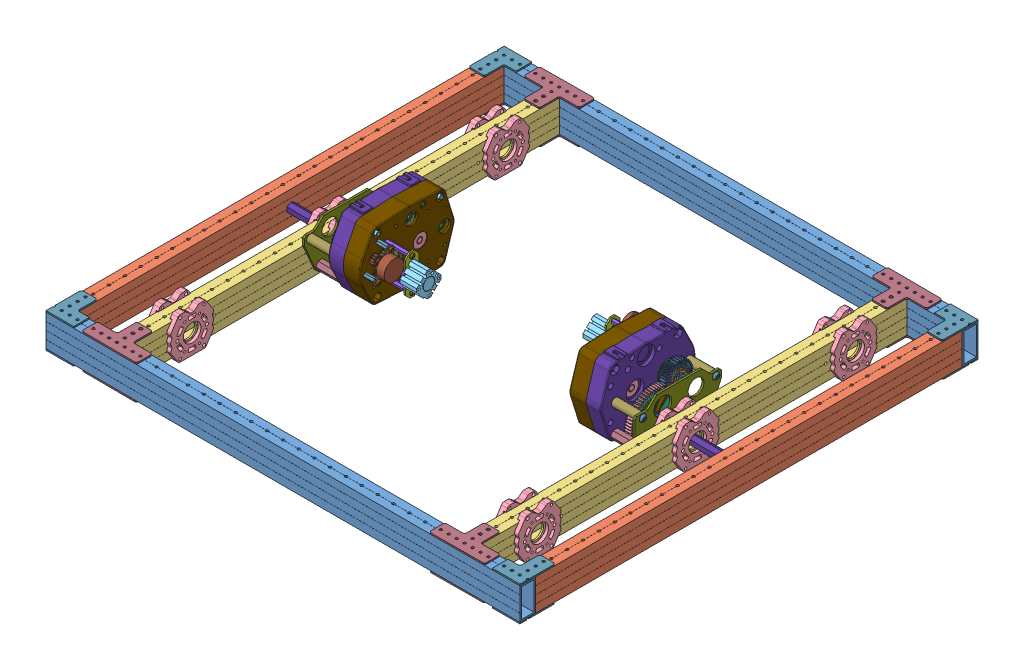
SolidWorks assembly Drivebase, configuration Default. Lengths in mm.
Overall size (762 166.93 737.13).
257 component instances, 69 part files, 0 mates.
Components (placement in the parent):
- 2020IR.drivebase.originaldownload.osears-1: 2020IR.drivebase.originaldownload.osears [Default] at (381 -50.8 -368.3) size (762 166.93 737.13)
  - 1_x_2_x_0_100_Pre-Drilled_VersaFrame_Aluminum_Tube_(30)_217-3453.drp-1: 1_x_2_x_0_100_Pre-Drilled_VersaFrame_Aluminum_Tube_(30)_217-3453.drp [Default] at (-12.7 25.4 12.7) x (0 0 -1) z (1 0 0) size (25.4 50.8 762)
  - 1_x_2_x_0_100_Pre-Drilled_VersaFrame_Aluminum_Tube_(27)_217-3453.drp-1: 1_x_2_x_0_100_Pre-Drilled_VersaFrame_Aluminum_Tube_(27)_217-3453.drp [Default] at (-12.7 25.4 774.7) size (25.4 50.8 685.8)
  - 1_x_2_x_0_100_Pre-Drilled_VersaFrame_Aluminum_Tube_(27)_217-3453.drp-2: 1_x_2_x_0_100_Pre-Drilled_VersaFrame_Aluminum_Tube_(27)_217-3453.drp [Default] at (-749.3 25.4 774.7) size (25.4 50.8 685.8)
  - 1_x_2_x_0_100_Pre-Drilled_VersaFrame_Aluminum_Tube_(30)_217-3453.drp-2: 1_x_2_x_0_100_Pre-Drilled_VersaFrame_Aluminum_Tube_(30)_217-3453.drp [Default] at (-749.3 25.4 723.9) x (0 0 1) z (-1 0 0) size (25.4 50.8 762)
  - Copy of 2020IR.subassembly_drivebase_gearbox_wheels_mounted.originaldownload.osears-1: Copy of 2020IR.subassembly_drivebase_gearbox_wheels_mounted.originaldownload.osears [Default] at (-647.7 2.54 25.4) size (265.36 166.93 685.8)
    - 217-8000-001-002_mod_to_1_x_2_x_0_100_Pre-Drilled_VersaFrame_Aluminum_Tube_(27)_217-3453.drp-1: 217-8000-001-002_mod_to_1_x_2_x_0_100_Pre-Drilled_VersaFrame_Aluminum_Tube_(27)_217-3453.drp [Default] at (-12.7 22.86 749.3) size (25.4 50.8 685.8)
    - VersaBlock_Kit_217-3432.drp-1: VersaBlock_Kit_217-3432.drp [Default] at (1.5875 24.5237 596.8746) x (0 0 -1) z (1 0 0) size (69.4 66.32 9.53)
    - VersaBlock_Kit_217-3432.drp-2: VersaBlock_Kit_217-3432.drp [Default] at (1.5875 24.5237 342.8746) x (0 0 -1) z (1 0 0) size (69.4 66.32 9.53)
    - VersaBlock_Kit_217-3432.drp-3: VersaBlock_Kit_217-3432.drp [Default] at (1.5875 24.5237 88.8746) x (0 0 -1) z (1 0 0) size (69.4 66.32 9.53)
    - VersaBlock_Kit_217-3432.drp-4: VersaBlock_Kit_217-3432.drp [Default] at (-26.9875 24.5237 88.8746) x (0 0 1) z (-1 0 0) size (69.4 66.32 9.53)
    - VersaBlock_Kit_217-3432.drp-5: VersaBlock_Kit_217-3432.drp [Default] at (-26.9875 24.5237 342.8746) x (0 0 1) z (-1 0 0) size (69.4 66.32 9.53)
    - VersaBlock_Kit_217-3432.drp-6: VersaBlock_Kit_217-3432.drp [Default] at (-26.9875 24.5237 596.8746) x (0 0 1) z (-1 0 0) size (69.4 66.32 9.53)
    - 3_CIM_Ball_Shifter_Base_Kit_with_WCD_3rd_Stage_217-3269_With_NEO.drp-1: 3_CIM_Ball_Shifter_Base_Kit_with_WCD_3rd_Stage_217-3269_With_NEO.drp [Default] at (101.2952 62.8142 378.4138) x (0 1 0) z (-1 0 0) size (166.93 180.09 265.36)
      - 3_CIM_Ball_Shifter_Base_Kit_with_WCD_3rd_Stage_217-3269.STEP-1: 3_CIM_Ball_Shifter_Base_Kit_with_WCD_3rd_Stage_217-3269.STEP [Default] at origin size (154.62 161.2 265.36)
        - 217-2778-001 Rev2_NCQ8A075-050M.STEP-1: 217-2778-001 Rev2_NCQ8A075-050M.STEP [Default] at (0 0 -53.848) x (-0.707107 0.707107 0) z (0 0 1) size (31.75 33.34 39.88)
          - 217-2778-NCQ8A075-050M_NCQ8 Tube_075A.STEP-1: 217-2778-NCQ8A075-050M_NCQ8 Tube_075A.STEP [Default] at origin size (31.75 33.34 26.92)
          - 217-2778-NCQ8A075-050M_NCQ8 Rod_075M.STEP-1: 217-2778-NCQ8A075-050M_NCQ8 Rod_075M.STEP [Default] at (0 0 -8.85) x (0.866025 -0.5 0) z (0 0 1) size (18.95 18.95 35.27)
          - 217-2778-NCQ8A075-050M_Snap Ring_075.STEP-1: 217-2778-NCQ8A075-050M_Snap Ring_075.STEP [Default] at (0 0 10.362) size (21 20.74 0.97)
        - 217-4098-100 Rev1.STEP-1: 217-4098-100 Rev1.STEP [Default] at (0 0 -16.927) x (-0.503316 0.864103 0) z (0 0 1) size (18.03 19.79 22.46)
          - 217-4098-006 Rev2.STEP-1: 217-4098-006 Rev2.STEP [Default] at (0 0 -4.6312) x (0 -1 0) z (0 0 -1) size (18.09 11.02 22.46)
          - 217-4098-006 Rev2.STEP-2: 217-4098-006 Rev2.STEP [Default] at (0 0 -4.6312) x (0 1 0) z (0 0 -1) size (18.09 11.02 22.46)
          - 217-3489-001 Rev1.STEP-1: 217-3489-001 Rev1.STEP [Default] at (0 0 -4.6312) x (0 0 1) z (-0.980217 -0.197926 0) size (4.77 12.7 12.7)
          - 97633A130_97633A130_grv.STEP-1: 97633A130_97633A130_grv.STEP [Default] at (0 0 -7.33) x (0 0 -1) z (0.979861 0.199683 0) size (0.64 8.74 7.34)
          - 91251A107_91251A107.STEP-1: 91251A107_91251A107.STEP [Default] at (-4.8375 -6.735 -9.4343) x (0 0.863883 -0.503692) z (-1 0 0) size (4.65 4.65 10.79)
          - 91251A107_91251A107.STEP-2: 91251A107_91251A107.STEP [Default] at (4.8375 6.735 -9.4343) x (0 0.470889 -0.882193) z (1 0 0) size (4.65 4.65 10.79)
        - 217-3288-001 Rev3.STEP-1: 217-3288-001 Rev3.STEP [Default] at (0 0 0.0889) x (0.055929 -0.998435 0) z (0 0 1) size (99.51 99.53 98.3)
          - 217-4099-000 Rev2_high gear.STEP-1: 217-4099-000 Rev2_high gear.STEP [Default] x (-1 0 0) z (0 0 1) size (22.23 22.23 98.3)
            - 217-4098-005 Rev1_91612A226.STEP-1: 217-4098-005 Rev1_91612A226.STEP [Default] at (0 0 46.2661) x (-0.144757 0 0.989467) z (0 -1 0) size (3.02 3.15 18.22)
            - 217-4098-003 Rev2.STEP-1: 217-4098-003 Rev2.STEP [Default] x (1 0 0) z (0 0 -1) size (22.23 22.23 55.94)
            - 217-4099-002 Rev3.STEP-1: 217-4099-002 Rev3.STEP [Default] at (0 0 53.467) x (0 0 1) z (-1 0 0) size (40.96 12.73 14.67)
            - 217-4098-004 Rev1.STEP-1: 217-4098-004 Rev1.STEP [Default] at (0 0 14.2494) x (0.873474 -0.48687 0) z (0 0 1) size (11.68 11.68 56)
          - 217-3212-101 Rev1.STEP-1: 217-3212-101 Rev1.STEP [Default] at (-11.5751 10.4131 45.3224) x (0.923728 0.383049 0) z (0 0 -1) size (46.46 46.56 12.7)
            - 217-2428-022 Rev1.STEP-1: 217-2428-022 Rev1.STEP [Default] at (6.7035 14.0527 24.6087) size (28.57 28.57 6.1)
            - 217-3212-001 Rev1_34t.STEP-1: 217-3212-001 Rev1_34t.STEP [Default] at (6.7035 14.0527 27.9107) size (46.46 46.56 11.11)
          - 217-3222-101 Rev1.STEP-1: 217-3222-101 Rev1.STEP [Default] at (21.0941 -5.2804 52.7371) x (-0.889163 -0.457591 0) z (0 0 -1) size (73.87 73.92 12.7)
            - 217-2428-022 Rev1.STEP-1: 217-2428-022 Rev1.STEP [Default] at (16.3398 14.3476 19.3234) size (28.57 28.57 6.1)
            - 217-3222-001 Rev1_Spur01.STEP-1: 217-3222-001 Rev1_Spur01.STEP [Default] at (16.3398 14.3476 22.6254) x (0.999377 0.0353 0) z (0 0 1) size (71.39 71.45 11.11)
          - 217-2428-008 Rev2.STEP-1: 217-2428-008 Rev2.STEP [Default] at (0 0 10.2679) size (31.75 31.75 1.59)
          - 217-2428-028 Rev1_97633A250.STEP-1: 217-2428-028 Rev1_97633A250.STEP [Default] at (0 0 37.1221) x (0 0 1) z (0.9357 -0.352797 0) size (1.07 23.39 21.18)
          - 217-2428-007 Rev1.STEP-1: 217-2428-007 Rev1.STEP [Default] at (7.809 4.5085 14.2494) x (-0.69071 0.455693 -0.561483) z (-0.67559 -0.683536 0.276329) size (6.35 6.35 6.35)
          - 217-2428-007 Rev1.STEP-2: 217-2428-007 Rev1.STEP [Default] at (5.4343 3.1375 26.9494) x (-0.162331 -0.978398 0.128005) z (0.857281 -0.204076 -0.472676) size (6.35 6.35 6.35)
          - 217-2428-007 Rev1.STEP-3: 217-2428-007 Rev1.STEP [Default] at (-5.4343 3.1375 26.9494) x (0.928483 0.348617 0.128005) z (-0.251905 0.844465 -0.472676) size (6.35 6.35 6.35)
          - 217-2428-007 Rev1.STEP-4: 217-2428-007 Rev1.STEP [Default] at (0 -6.275 26.9494) x (-0.766153 0.629782 0.128005) z (-0.605376 -0.640389 -0.472676) size (6.35 6.35 6.35)
          - 217-2428-007 Rev1.STEP-5: 217-2428-007 Rev1.STEP [Default] at (-7.809 4.5085 14.2494) x (-0.049287 -0.826019 -0.561483) z (0.929754 -0.24331 0.276329) size (6.35 6.35 6.35)
          - 217-2428-007 Rev1.STEP-6: 217-2428-007 Rev1.STEP [Default] at (0 -9.017 14.2494) x (0.739997 0.370326 -0.561483) z (-0.254164 0.926846 0.276329) size (6.35 6.35 6.35)
        - 217-2733-001 Rev2.STEP-1: 217-2733-001 Rev2.STEP [Default] at (0 53.4162 37.6682) x (0 0 1) z (-0.00054 -1 0) size (7.11 24.61 24.61)
        - 217-2733-001 Rev2.STEP-2: 217-2733-001 Rev2.STEP [Default] at (0 53.4162 7.9248) x (0 0 -1) z (-0.038475 0.99926 0) size (7.11 24.61 24.61)
        - 217-2731-001 Rev2.STEP-1: 217-2731-001 Rev2.STEP [Default] at (0 0 0.0381) x (-0.099212 0.995066 0) z (0.995066 0.099212 0) size (31.12 7.94 31.12)
        - 217-2789-001 Rev2.STEP-1: 217-2789-001 Rev2.STEP [Default] at (0 0 43.2943) x (0 0 -1) z (-0.58471 0.811243 0) size (11.1 38.4 38.4)
        - 217-2428-012 Rev2.STEP-1: 217-2428-012 Rev2.STEP [Default] at (0 0 -40.386) size (63.5 22.23 2.29)
        - 217-2428-005 Rev1.STEP-1: 217-2428-005 Rev1.STEP [Default] at (25.4 0 -19.05) x (-0.557362 -0.83027 0) z (-0.83027 0.557362 0) size (7.33 38.98 6.35)
        - 217-2428-005 Rev1.STEP-2: 217-2428-005 Rev1.STEP [Default] at (-25.4 0 -19.05) x (0.667436 0.744667 0) z (0.744667 -0.667436 0) size (7.33 38.98 6.35)
        - SCREW-832-0375.STEP-1: SCREW-832-0375.STEP [Default] at (25.4 0 -42.5958) x (0 0 1) z (-0.875404 0.483392 0) size (11.73 7.92 7.92)
        - SCREW-832-0375.STEP-2: SCREW-832-0375.STEP [Default] at (-25.4 0 -42.5958) x (0 0 1) z (-0.966319 0.257347 0) size (11.73 7.92 7.92)
        - SCREW-832-0375.STEP-3: SCREW-832-0375.STEP [Default] at (25.4 0 5.3848) x (0 0 -1) z (1 0 0) size (11.73 7.92 7.92)
        - SCREW-832-0375.STEP-4: SCREW-832-0375.STEP [Default] at (-25.4 0 5.3848) x (0 0 -1) z (0.941463 -0.337115 0) size (11.73 7.92 7.92)
        - SBS1_SBS-0632-0250.STEP-1: SBS1_SBS-0632-0250.STEP [Default] at (15.494 0 -36.2458) x (0 0 -1) z (0.854303 -0.519775 0) size (8.57 6.68 6.65)
        - SBS1_SBS-0632-0250.STEP-2: SBS1_SBS-0632-0250.STEP [Default] at (-15.494 0 -36.2458) x (0 0 -1) z (0.854303 -0.519775 0) size (8.57 6.68 6.65)
        - 217-2428-017 Rev2.STEP-1: 217-2428-017 Rev2.STEP [Default] at (12.7 -21.997 -3.614) x (-0.578458 -0.815712 0) z (0 0 -1) size (14.73 14.73 7.37)
        - 217-2428-016 Rev3_Spur01.STEP-1: 217-2428-016 Rev3_Spur01.STEP [Default] at (0 0 -3.614) x (0.873157 -0.48744 0) z (0 0 1) size (40.67 40.74 13.32)
        - 217-2428-019 Rev1.STEP-1: 217-2428-019 Rev1.STEP [Default] at (12.7 -21.997 -20.6248) x (0.866025 0.5 0) z (0 0 1) size (50.8 19.05 1.57)
        - 217-2428-006 Rev1.STEP-1: 217-2428-006 Rev1.STEP [Default] at (32.079 -14.2875 -9.525) x (-0.752416 0.658689 0) z (0.658689 0.752416 0) size (7.33 19.93 6.35)
        - 217-2428-006 Rev1.STEP-2: 217-2428-006 Rev1.STEP [Default] at (-3.6662 -34.925 -9.525) x (0.84498 0.534798 0) z (0.534798 -0.84498 0) size (7.33 19.93 6.35)
        - SCREW-832-0375.STEP-5: SCREW-832-0375.STEP [Default] at (32.079 -14.2875 4.7498) x (0 0 -1) z (0.980613 0.195955 0) size (11.73 7.92 7.92)
        - SCREW-832-0375.STEP-6: SCREW-832-0375.STEP [Default] at (-3.6662 -34.925 5.3848) x (0 0 -1) z (-0.672515 -0.740083 0) size (11.73 7.92 7.92)
        - SCREW-832-0375.STEP-7: SCREW-832-0375.STEP [Default] at (-3.6662 -34.925 -22.8346) x (0 0 1) z (0.948865 0.315681 0) size (11.73 7.92 7.92)
        - SCREW-832-0375.STEP-8: SCREW-832-0375.STEP [Default] at (32.079 -14.2875 -22.8346) x (0 0 1) z (-0.875404 0.483392 0) size (11.73 7.92 7.92)
        - 217-2614-001_12t.STEP-1: 217-2614-001_12t.STEP [Default] at (36.9798 39.6868 15.8623) x (-0.087156 0.996195 0) z (0 0 1) size (18.29 18.29 19)
        - 217-2761-001 rev1.STEP-1: 217-2761-001 rev1.STEP [Default] at (33.1943 39.3556 16.1) x (0.087156 -0.996195 0) z (0 0 1) size (2 2 20)
        - 217-2761-001 rev1.STEP-2: 217-2761-001 rev1.STEP [Default] at (-40.7653 40.018 16.1) x (0.087156 0.996195 0) z (0 0 1) size (2 2 20)
        - 217-2614-001_12t.STEP-2: 217-2614-001_12t.STEP [Default] at (-36.9798 39.6868 15.8623) x (0.087156 0.996195 0) z (0 0 1) size (18.29 18.29 19)
        - 217-2614-001_12t.STEP-3: 217-2614-001_12t.STEP [Default] at (0 92.8624 15.8623) x (0.97459 0.223996 0) z (0 0 1) size (18.29 18.29 19)
        - 217-2761-001 rev1.STEP-3: 217-2761-001 rev1.STEP [Default] at (-0.8512 96.5658 16.1) x (0.97459 0.223996 0) z (0 0 1) size (2 2 20)
        - 217-3195-002 rev2.STEP-1: 217-3195-002 rev2.STEP [Default] at (0 0 50.546) x (-1 0 0) z (0 0 -1) size (114.31 152.24 24.96)
        - 217-3195-001 Rev1.STEP-1: 217-3195-001 Rev1.STEP [Default] at origin size (113.41 152.24 26.86)
        - Nylock Nut_NNY2520-ZC.STEP-1: Nylock Nut_NNY2520-ZC.STEP [Default] at (48.8823 73.025 37.846) x (0 0.866025 -0.5) z (-1 0 0) size (12.85 11.89 7.62)
        - Nylock Nut_NNY2520-ZC.STEP-2: Nylock Nut_NNY2520-ZC.STEP [Default] at (48.8823 -3.175 37.846) x (0 0 -1) z (-1 0 0) size (12.85 11.89 7.62)
        - Nylock Nut_NNY2520-ZC.STEP-3: Nylock Nut_NNY2520-ZC.STEP [Default] at (44.45 85.725 7.8613) x (0 1 0) z (0 0 -1) size (12.85 11.89 7.62)
        - 276-1027-001.STEP-1: 276-1027-001.STEP [Default] at (47.625 58.1787 6.35) x (0 1 0) z (-1 0 0) size (8.61 5.64 9.94)
        - 276-1027-001.STEP-2: 276-1027-001.STEP [Default] at (-47.625 58.1787 6.35) x (0 -1 0) z (1 0 0) size (8.61 5.64 9.94)
        - SCREW-832-1750.STEP-1: SCREW-832-1750.STEP [Default] at (-47.625 58.1787 47.0408) x (0 0 -1) z (-0.960822 -0.277167 0) size (46.66 7.92 7.92)
        - SCREW-832-1750.STEP-2: SCREW-832-1750.STEP [Default] at (47.625 58.1787 47.0408) x (0 0 -1) z (-0.960822 -0.277167 0) size (46.66 7.92 7.92)
        - Nylock Nut_NNY2520-ZC.STEP-4: Nylock Nut_NNY2520-ZC.STEP [Default] at (44.45 -15.875 7.8613) x (0 1 0) z (0 0 -1) size (12.85 11.89 7.62)
        - 217-2428-004 Rev3.STEP-1: 217-2428-004 Rev3.STEP [Default] at (0 53.4162 22.7711) x (-0.709585 0.70462 0) z (0 0 1) size (11 9.53 43.92)
        - SBS1_SBS-2520-1625SS.STEP-1: SBS1_SBS-2520-1625SS.STEP [Default] at (44.45 85.725 42.4688) x (0 0 -1) z (-0.251219 0.96793 0) size (45.3 11.2 11.18)
        - SBS1_SBS-2520-1625SS.STEP-2: SBS1_SBS-2520-1625SS.STEP [Default] at (44.45 -15.875 42.4688) x (0 0 -1) z (-0.251219 0.96793 0) size (45.3 11.2 11.18)
        - SBS1_SBS2520-1750.STEP-1: SBS1_SBS2520-1750.STEP [Default] at (-44.45 85.725 7.4422) x (0 0 1) z (-0.031478 0.999504 0) size (48.48 11.2 11.18)
        - SBS1_SBS2520-1750.STEP-2: SBS1_SBS2520-1750.STEP [Default] at (-44.45 -15.875 7.4422) x (0 0 1) z (-0.937114 -0.349025 0) size (48.48 11.2 11.18)
        - 217-2428-021 Rev1.STEP-1: 217-2428-021 Rev1.STEP [Default] at (0 53.4162 9.5123) x (0.451333 -0.892356 0) z (0 0 1) size (15.88 15.88 3.17)
        - 217-2428-029 Rev1.STEP-1: 217-2428-029 Rev1.STEP [Default] at (0 53.4162 36.957) x (0.999846 0.017557 0) z (0 0 1) size (15.88 15.88 1.12)
        - Grayhill Lock Washer.STEP-1: Grayhill Lock Washer.STEP [Default] at (12.7 -21.997 -18.6817) x (0.467173 -0.884166 0) z (0 0 1) size (19.69 19.69 0.74)
        - Grayhill Nut.STEP-1: Grayhill Nut.STEP [Default] at (12.7 -21.997 -17.0434) x (0.984088 0.177684 0) z (0 0 1) size (18.33 15.88 2.54)
        - Grahill Encoder.STEP-1: Grahill Encoder.STEP [Default] at (12.7 -21.997 -16.1798) x (-0.580071 0.814566 0) z (-0.814566 -0.580071 0) size (31.75 31.12 31.75)
        - 217-3195-009 Rev1_wcd 2.STEP-1: 217-3195-009 Rev1_wcd 2.STEP [Default] at (0 85.725 50.546) x (-0.998427 -0.056065 0) z (0 0 1) size (12.7 12.7 41.27)
        - 217-3195-006 Rev1_WCD.STEP-1: 217-3195-006 Rev1_WCD.STEP [Default] at (-44.45 85.725 44.1452) x (0.5 0.866025 0) z (0 0 1) size (12.7 14.66 47.62)
        - 217-3195-009 Rev1_wcd 2.STEP-2: 217-3195-009 Rev1_wcd 2.STEP [Default] at (0 -31.75 50.546) x (0.947633 0.319361 0) z (0 0 1) size (12.7 12.7 41.27)
        - 217-3195-006 Rev1_WCD.STEP-2: 217-3195-006 Rev1_WCD.STEP [Default] at (-44.45 -15.875 44.1452) x (0.5 -0.866025 0) z (0 0 1) size (12.7 14.66 47.62)
        - Nylock Nut_NNY2520-ZC.STEP-5: Nylock Nut_NNY2520-ZC.STEP [Default] at (0 -31.75 45.0723) x (-0.5 0.866025 0) z (0 0 -1) size (12.85 11.89 7.62)
        - Nylock Nut_NNY2520-ZC.STEP-6: Nylock Nut_NNY2520-ZC.STEP [Default] at (0 85.725 45.0723) x (-0.5 0.866025 0) z (0 0 -1) size (12.85 11.89 7.62)
        - SBS1_SBS-2520-2250.STEP-1: SBS1_SBS-2520-2250.STEP [Default] at (0 -31.75 98.298) x (0 0 -1) z (-0.933488 -0.358607 0) size (61.18 11.22 11.17)
        - SBS1_SBS2520-0625ZC.STEP-1: SBS1_SBS2520-0625ZC.STEP [Default] at (-44.45 85.725 98.298) x (0 0 -1) z (0.400817 0.916158 0) size (19.57 11.22 11.17)
        - SBS1_SBS2520-0625ZC.STEP-2: SBS1_SBS2520-0625ZC.STEP [Default] at (-44.45 -15.875 98.298) x (0 0 -1) z (-0.75178 -0.659414 0) size (19.57 11.22 11.17)
        - SBS1_SBS-2520-2250.STEP-2: SBS1_SBS-2520-2250.STEP [Default] at (0 85.725 98.298) x (0 0 -1) z (0.056677 -0.998393 0) size (61.18 11.22 11.17)
        - 217-3195-003 rev2.STEP-1: 217-3195-003 rev2.STEP [Default] at (0 0 94.9452) size (88.62 139.7 3.17)
        - 217-2617-003 Rev1.STEP-1: 217-2617-003 Rev1.STEP [Default] at (-39.878 35.5392 121.8535) x (-0.5 -0.866025 0) z (0 0 1) size (14.66 12.7 152.4)
        - 217-3109-001 Rev1.STEP-1: 217-3109-001 Rev1.STEP [Default] at (-39.878 35.5392 49.1808) x (0 0 1) z (0.312889 -0.94979 0) size (7.94 28.57 28.57)
        - 217-2734-001 Rev3.STEP-1: 217-2734-001 Rev3.STEP [Default] at (-39.878 35.5392 98.1202) x (1 0 0) z (0 1 0) size (31.12 7.94 31.12)
        - 217-2617-004 Rev1_97431A340_grv.STEP-1: 217-2617-004 Rev1_97431A340_grv.STEP [Default] at (-39.878 35.5392 54.8961) x (0 0 1) z (-0.124043 -0.992277 0) size (1.07 20.42 18.58)
        - 217-2617-004 Rev1_97431A340_grv.STEP-2: 217-2617-004 Rev1_97431A340_grv.STEP [Default] at (0 0 69.215) x (0 0 1) z (-0.124043 -0.992277 0) size (1.07 20.42 18.58)
        - 217-2702-001_20t.STEP-1: 217-2702-001_20t.STEP [Default] at (0 0 62.357) x (0.998435 0.055929 0) z (0 0 1) size (28.2 28.2 12.65)
        - 217-2715-002 Rev1_64t.STEP-1: 217-2715-002 Rev1_64t.STEP [Default] at (-39.878 35.5392 61.7541) x (0.866025 -0.5 0) z (0 0 1) size (84.3 84.3 12.65)
        - 217-2704-001_24.STEP-1: 217-2704-001_24.STEP [Default] at (0 0 62.357) x (0.450781 0.892635 0) z (0 0 -1) size (33.29 33.29 12.65)
        - 217-2714-002 Rev1_60t.STEP-1: 217-2714-002 Rev1_60t.STEP [Default] at (-39.878 35.5392 61.7541) x (0.866025 -0.5 0) z (0 0 1) size (78.95 78.95 12.65)
        - 217-3221-002 Rev1.STEP-1: 217-3221-002 Rev1.STEP [Default] at (-39.878 35.5392 61.7414) x (0 -1 0) z (0 0 1) size (71.39 71.45 12.62)
        - 217-2705-001_30t.STEP-1: 217-2705-001_30t.STEP [Default] at (0 0 62.357) x (0.547654 -0.836705 0) z (0 0 1) size (41.01 41.12 12.65)
        - 217-2712-002 Rev1_50t.STEP-1: 217-2712-002 Rev1_50t.STEP [Default] at (-39.878 35.5392 61.7541) x (0.866025 -0.5 0) z (0 0 1) size (66.7 66.76 12.65)
        - 217-2706-001_34t.STEP-1: 217-2706-001_34t.STEP [Default] at (0 0 62.357) x (0.998435 0.055929 0) z (0 0 1) size (46.46 46.56 12.65)
        - 217-3210-001 Rev1_30t.STEP-1: 217-3210-001 Rev1_30t.STEP [Default] at (0 53.4162 30.0736) x (-0.966828 0.255427 0) z (0 0 1) size (41.01 41.12 12.65)
        - 217-2711-002 Rev1_50t.STEP-1: 217-2711-002 Rev1_50t.STEP [Default] at (0 53.4162 17.4244) x (0.262208 -0.965011 0) z (0 0 1) size (66.7 66.76 12.65)
      - REV-21-1650 (1).step-1: REV-21-1650 (1).step [Default] at (0 92.8624 0) size (64.41 64.76 93.26)
      - REV-21-1650 (1).step-2: REV-21-1650 (1).step [Default] at (36.9798 39.6868 0) x (0.996195 0.087156 0) z (0 0 1) size (64.41 64.76 93.26)
      - REV-21-1650 (1).step-3: REV-21-1650 (1).step [Default] at (-36.9798 39.6868 0) x (0.996195 -0.087156 0) z (0 0 1) size (64.41 64.76 93.26)
  - Copy of 2020IR.subassembly_drivebase_gearbox_wheels_mounted.originaldownload.osears_2-1: Copy of 2020IR.subassembly_drivebase_gearbox_wheels_mounted.originaldownload.osears_2 [Default] at (-114.3 2.54 711.2) x (-1 0 0) z (0 0 -1) size (265.36 166.93 685.8)
    - 217-8000-001-002_mod_to_1_x_2_x_0_100_Pre-Drilled_VersaFrame_Aluminum_Tube_(27)_217-3453.drp-1: 217-8000-001-002_mod_to_1_x_2_x_0_100_Pre-Drilled_VersaFrame_Aluminum_Tube_(27)_217-3453.drp [Default] at (-12.7 22.86 749.3) size (25.4 50.8 685.8)
    - VersaBlock_Kit_217-3432.drp-1: VersaBlock_Kit_217-3432.drp [Default] at (1.5875 24.5237 596.8746) x (0 0 -1) z (1 0 0) size (69.4 66.32 9.53)
    - VersaBlock_Kit_217-3432.drp-2: VersaBlock_Kit_217-3432.drp [Default] at (1.5875 24.5237 342.8746) x (0 0 -1) z (1 0 0) size (69.4 66.32 9.53)
    - VersaBlock_Kit_217-3432.drp-3: VersaBlock_Kit_217-3432.drp [Default] at (1.5875 24.5237 88.8746) x (0 0 -1) z (1 0 0) size (69.4 66.32 9.53)
    - VersaBlock_Kit_217-3432.drp-4: VersaBlock_Kit_217-3432.drp [Default] at (-26.9875 24.5237 88.8746) x (0 0 1) z (-1 0 0) size (69.4 66.32 9.53)
    - VersaBlock_Kit_217-3432.drp-5: VersaBlock_Kit_217-3432.drp [Default] at (-26.9875 24.5237 342.8746) x (0 0 1) z (-1 0 0) size (69.4 66.32 9.53)
    - VersaBlock_Kit_217-3432.drp-6: VersaBlock_Kit_217-3432.drp [Default] at (-26.9875 24.5237 596.8746) x (0 0 1) z (-1 0 0) size (69.4 66.32 9.53)
    - 3_CIM_Ball_Shifter_Base_Kit_with_WCD_3rd_Stage_217-3269_With_NEO.drp_2-1: 3_CIM_Ball_Shifter_Base_Kit_with_WCD_3rd_Stage_217-3269_With_NEO.drp_2 [Default] at (101.2952 62.8142 378.4138) x (0 1 0) z (-1 0 0) size (166.93 180.09 265.36)
      - 3_CIM_Ball_Shifter_Base_Kit_with_WCD_3rd_Stage_217-3269.STEP_2-1: 3_CIM_Ball_Shifter_Base_Kit_with_WCD_3rd_Stage_217-3269.STEP_2 [Default] at origin size (154.62 161.2 265.36)
        - 217-2778-001 Rev2_NCQ8A075-050M.STEP_2-1: 217-2778-001 Rev2_NCQ8A075-050M.STEP_2 [Default] at (0 0 -53.848) x (-0.707107 0.707107 0) z (0 0 1) size (31.75 33.34 39.88)
          - 217-2778-NCQ8A075-050M_NCQ8 Tube_075A.STEP-1: 217-2778-NCQ8A075-050M_NCQ8 Tube_075A.STEP [Default] at origin size (31.75 33.34 26.92)
          - 217-2778-NCQ8A075-050M_NCQ8 Rod_075M.STEP-1: 217-2778-NCQ8A075-050M_NCQ8 Rod_075M.STEP [Default] at (0 0 -8.85) x (0.866025 -0.5 0) z (0 0 1) size (18.95 18.95 35.27)
          - 217-2778-NCQ8A075-050M_Snap Ring_075.STEP-1: 217-2778-NCQ8A075-050M_Snap Ring_075.STEP [Default] at (0 0 10.362) size (21 20.74 0.97)
        - 217-4098-100 Rev1.STEP_2-1: 217-4098-100 Rev1.STEP_2 [Default] at (0 0 -16.927) x (-0.503316 0.864103 0) z (0 0 1) size (18.03 19.79 22.46)
          - 217-4098-006 Rev2.STEP-1: 217-4098-006 Rev2.STEP [Default] at (0 0 -4.6312) x (0 -1 0) z (0 0 -1) size (18.09 11.02 22.46)
          - 217-4098-006 Rev2.STEP-2: 217-4098-006 Rev2.STEP [Default] at (0 0 -4.6312) x (0 1 0) z (0 0 -1) size (18.09 11.02 22.46)
          - 217-3489-001 Rev1.STEP-1: 217-3489-001 Rev1.STEP [Default] at (0 0 -4.6312) x (0 0 1) z (-0.980217 -0.197926 0) size (4.77 12.7 12.7)
          - 97633A130_97633A130_grv.STEP-1: 97633A130_97633A130_grv.STEP [Default] at (0 0 -7.33) x (0 0 -1) z (0.979861 0.199683 0) size (0.64 8.74 7.34)
          - 91251A107_91251A107.STEP-1: 91251A107_91251A107.STEP [Default] at (-4.8375 -6.735 -9.4343) x (0 0.863883 -0.503692) z (-1 0 0) size (4.65 4.65 10.79)
          - 91251A107_91251A107.STEP-2: 91251A107_91251A107.STEP [Default] at (4.8375 6.735 -9.4343) x (0 0.470889 -0.882193) z (1 0 0) size (4.65 4.65 10.79)
        - 217-3288-001 Rev3.STEP_2-1: 217-3288-001 Rev3.STEP_2 [Default] at (0 0 0.0889) x (0.055929 -0.998435 0) z (0 0 1) size (99.51 99.53 98.3)
          - 217-4099-000 Rev2_high gear.STEP_2-1: 217-4099-000 Rev2_high gear.STEP_2 [Default] x (-1 0 0) z (0 0 1) size (22.23 22.23 98.3)
            - 217-4098-005 Rev1_91612A226.STEP-1: 217-4098-005 Rev1_91612A226.STEP [Default] at (0 0 46.2661) x (-0.144757 0 0.989467) z (0 -1 0) size (3.02 3.15 18.22)
            - 217-4098-003 Rev2.STEP-1: 217-4098-003 Rev2.STEP [Default] x (1 0 0) z (0 0 -1) size (22.23 22.23 55.94)
            - 217-4099-002 Rev3.STEP-1: 217-4099-002 Rev3.STEP [Default] at (0 0 53.467) x (0 0 1) z (-1 0 0) size (40.96 12.73 14.67)
            - 217-4098-004 Rev1.STEP-1: 217-4098-004 Rev1.STEP [Default] at (0 0 14.2494) x (0.873474 -0.48687 0) z (0 0 1) size (11.68 11.68 56)
          - 217-3212-101 Rev1.STEP_2-1: 217-3212-101 Rev1.STEP_2 [Default] at (-11.5751 10.4131 45.3224) x (0.923728 0.383049 0) z (0 0 -1) size (46.46 46.56 12.7)
            - 217-2428-022 Rev1.STEP-1: 217-2428-022 Rev1.STEP [Default] at (6.7035 14.0527 24.6087) size (28.57 28.57 6.1)
            - 217-3212-001 Rev1_34t.STEP-1: 217-3212-001 Rev1_34t.STEP [Default] at (6.7035 14.0527 27.9107) size (46.46 46.56 11.11)
          - 217-3222-101 Rev1.STEP_2-1: 217-3222-101 Rev1.STEP_2 [Default] at (21.0941 -5.2804 52.7371) x (-0.889163 -0.457591 0) z (0 0 -1) size (73.87 73.92 12.7)
            - 217-2428-022 Rev1.STEP-1: 217-2428-022 Rev1.STEP [Default] at (16.3398 14.3476 19.3234) size (28.57 28.57 6.1)
            - 217-3222-001 Rev1_Spur01.STEP-1: 217-3222-001 Rev1_Spur01.STEP [Default] at (16.3398 14.3476 22.6254) x (0.999377 0.0353 0) z (0 0 1) size (71.39 71.45 11.11)
          - 217-2428-008 Rev2.STEP-1: 217-2428-008 Rev2.STEP [Default] at (0 0 10.2679) size (31.75 31.75 1.59)
          - 217-2428-028 Rev1_97633A250.STEP-1: 217-2428-028 Rev1_97633A250.STEP [Default] at (0 0 37.1221) x (0 0 1) z (0.9357 -0.352797 0) size (1.07 23.39 21.18)
          - 217-2428-007 Rev1.STEP-1: 217-2428-007 Rev1.STEP [Default] at (7.809 4.5085 14.2494) x (-0.69071 0.455693 -0.561483) z (-0.67559 -0.683536 0.276329) size (6.35 6.35 6.35)
          - 217-2428-007 Rev1.STEP-2: 217-2428-007 Rev1.STEP [Default] at (5.4343 3.1375 26.9494) x (-0.162331 -0.978398 0.128005) z (0.857281 -0.204076 -0.472676) size (6.35 6.35 6.35)
          - 217-2428-007 Rev1.STEP-3: 217-2428-007 Rev1.STEP [Default] at (-5.4343 3.1375 26.9494) x (0.928483 0.348617 0.128005) z (-0.251905 0.844465 -0.472676) size (6.35 6.35 6.35)
          - 217-2428-007 Rev1.STEP-4: 217-2428-007 Rev1.STEP [Default] at (0 -6.275 26.9494) x (-0.766153 0.629782 0.128005) z (-0.605376 -0.640389 -0.472676) size (6.35 6.35 6.35)
          - 217-2428-007 Rev1.STEP-5: 217-2428-007 Rev1.STEP [Default] at (-7.809 4.5085 14.2494) x (-0.049287 -0.826019 -0.561483) z (0.929754 -0.24331 0.276329) size (6.35 6.35 6.35)
          - 217-2428-007 Rev1.STEP-6: 217-2428-007 Rev1.STEP [Default] at (0 -9.017 14.2494) x (0.739997 0.370326 -0.561483) z (-0.254164 0.926846 0.276329) size (6.35 6.35 6.35)
        - 217-2733-001 Rev2.STEP-1: 217-2733-001 Rev2.STEP [Default] at (0 53.4162 37.6682) x (0 0 1) z (-0.00054 -1 0) size (7.11 24.61 24.61)
        - 217-2733-001 Rev2.STEP-2: 217-2733-001 Rev2.STEP [Default] at (0 53.4162 7.9248) x (0 0 -1) z (-0.038475 0.99926 0) size (7.11 24.61 24.61)
        - 217-2731-001 Rev2.STEP-1: 217-2731-001 Rev2.STEP [Default] at (0 0 0.0381) x (-0.099212 0.995066 0) z (0.995066 0.099212 0) size (31.12 7.94 31.12)
        - 217-2789-001 Rev2.STEP-1: 217-2789-001 Rev2.STEP [Default] at (0 0 43.2943) x (0 0 -1) z (-0.58471 0.811243 0) size (11.1 38.4 38.4)
        - 217-2428-012 Rev2.STEP-1: 217-2428-012 Rev2.STEP [Default] at (0 0 -40.386) size (63.5 22.23 2.29)
        - 217-2428-005 Rev1.STEP-1: 217-2428-005 Rev1.STEP [Default] at (25.4 0 -19.05) x (-0.557362 -0.83027 0) z (-0.83027 0.557362 0) size (7.33 38.98 6.35)
        - 217-2428-005 Rev1.STEP-2: 217-2428-005 Rev1.STEP [Default] at (-25.4 0 -19.05) x (0.667436 0.744667 0) z (0.744667 -0.667436 0) size (7.33 38.98 6.35)
        - SCREW-832-0375.STEP-1: SCREW-832-0375.STEP [Default] at (25.4 0 -42.5958) x (0 0 1) z (-0.875404 0.483392 0) size (11.73 7.92 7.92)
        - SCREW-832-0375.STEP-2: SCREW-832-0375.STEP [Default] at (-25.4 0 -42.5958) x (0 0 1) z (-0.966319 0.257347 0) size (11.73 7.92 7.92)
        - SCREW-832-0375.STEP-3: SCREW-832-0375.STEP [Default] at (25.4 0 5.3848) x (0 0 -1) z (1 0 0) size (11.73 7.92 7.92)
        - SCREW-832-0375.STEP-4: SCREW-832-0375.STEP [Default] at (-25.4 0 5.3848) x (0 0 -1) z (0.941463 -0.337115 0) size (11.73 7.92 7.92)
        - SBS1_SBS-0632-0250.STEP-1: SBS1_SBS-0632-0250.STEP [Default] at (15.494 0 -36.2458) x (0 0 -1) z (0.854303 -0.519775 0) size (8.57 6.68 6.65)
        - SBS1_SBS-0632-0250.STEP-2: SBS1_SBS-0632-0250.STEP [Default] at (-15.494 0 -36.2458) x (0 0 -1) z (0.854303 -0.519775 0) size (8.57 6.68 6.65)
        - 217-2428-017 Rev2.STEP-1: 217-2428-017 Rev2.STEP [Default] at (12.7 -21.997 -3.614) x (-0.578458 -0.815712 0) z (0 0 -1) size (14.73 14.73 7.37)
        - 217-2428-016 Rev3_Spur01.STEP-1: 217-2428-016 Rev3_Spur01.STEP [Default] at (0 0 -3.614) x (0.873157 -0.48744 0) z (0 0 1) size (40.67 40.74 13.32)
        - 217-2428-019 Rev1.STEP-1: 217-2428-019 Rev1.STEP [Default] at (12.7 -21.997 -20.6248) x (0.866025 0.5 0) z (0 0 1) size (50.8 19.05 1.57)
        - 217-2428-006 Rev1.STEP-1: 217-2428-006 Rev1.STEP [Default] at (32.079 -14.2875 -9.525) x (-0.752416 0.658689 0) z (0.658689 0.752416 0) size (7.33 19.93 6.35)
        - 217-2428-006 Rev1.STEP-2: 217-2428-006 Rev1.STEP [Default] at (-3.6662 -34.925 -9.525) x (0.84498 0.534798 0) z (0.534798 -0.84498 0) size (7.33 19.93 6.35)
        - SCREW-832-0375.STEP-5: SCREW-832-0375.STEP [Default] at (32.079 -14.2875 4.7498) x (0 0 -1) z (0.980613 0.195955 0) size (11.73 7.92 7.92)
        - SCREW-832-0375.STEP-6: SCREW-832-0375.STEP [Default] at (-3.6662 -34.925 5.3848) x (0 0 -1) z (-0.672515 -0.740083 0) size (11.73 7.92 7.92)
        - SCREW-832-0375.STEP-7: SCREW-832-0375.STEP [Default] at (-3.6662 -34.925 -22.8346) x (0 0 1) z (0.948865 0.315681 0) size (11.73 7.92 7.92)
        - SCREW-832-0375.STEP-8: SCREW-832-0375.STEP [Default] at (32.079 -14.2875 -22.8346) x (0 0 1) z (-0.875404 0.483392 0) size (11.73 7.92 7.92)
        - 217-2614-001_12t.STEP-1: 217-2614-001_12t.STEP [Default] at (36.9798 39.6868 15.8623) x (-0.087156 0.996195 0) z (0 0 1) size (18.29 18.29 19)
        - 217-2761-001 rev1.STEP-1: 217-2761-001 rev1.STEP [Default] at (33.1943 39.3556 16.1) x (0.087156 -0.996195 0) z (0 0 1) size (2 2 20)
        - 217-2761-001 rev1.STEP-2: 217-2761-001 rev1.STEP [Default] at (-40.7653 40.018 16.1) x (0.087156 0.996195 0) z (0 0 1) size (2 2 20)
        - 217-2614-001_12t.STEP-2: 217-2614-001_12t.STEP [Default] at (-36.9798 39.6868 15.8623) x (0.087156 0.996195 0) z (0 0 1) size (18.29 18.29 19)
        - 217-2614-001_12t.STEP-3: 217-2614-001_12t.STEP [Default] at (0 92.8624 15.8623) x (0.97459 0.223996 0) z (0 0 1) size (18.29 18.29 19)
        - 217-2761-001 rev1.STEP-3: 217-2761-001 rev1.STEP [Default] at (-0.8512 96.5658 16.1) x (0.97459 0.223996 0) z (0 0 1) size (2 2 20)
        - 217-3195-002 rev2.STEP-1: 217-3195-002 rev2.STEP [Default] at (0 0 50.546) x (-1 0 0) z (0 0 -1) size (114.31 152.24 24.96)
        - 217-3195-001 Rev1.STEP-1: 217-3195-001 Rev1.STEP [Default] at origin size (113.41 152.24 26.86)
        - Nylock Nut_NNY2520-ZC.STEP-1: Nylock Nut_NNY2520-ZC.STEP [Default] at (48.8823 73.025 37.846) x (0 0.866025 -0.5) z (-1 0 0) size (12.85 11.89 7.62)
        - Nylock Nut_NNY2520-ZC.STEP-2: Nylock Nut_NNY2520-ZC.STEP [Default] at (48.8823 -3.175 37.846) x (0 0 -1) z (-1 0 0) size (12.85 11.89 7.62)
        - Nylock Nut_NNY2520-ZC.STEP-3: Nylock Nut_NNY2520-ZC.STEP [Default] at (44.45 85.725 7.8613) x (0 1 0) z (0 0 -1) size (12.85 11.89 7.62)
        - 276-1027-001.STEP-1: 276-1027-001.STEP [Default] at (47.625 58.1787 6.35) x (0 1 0) z (-1 0 0) size (8.61 5.64 9.94)
        - 276-1027-001.STEP-2: 276-1027-001.STEP [Default] at (-47.625 58.1787 6.35) x (0 -1 0) z (1 0 0) size (8.61 5.64 9.94)
        - SCREW-832-1750.STEP-1: SCREW-832-1750.STEP [Default] at (-47.625 58.1787 47.0408) x (0 0 -1) z (-0.960822 -0.277167 0) size (46.66 7.92 7.92)
        - SCREW-832-1750.STEP-2: SCREW-832-1750.STEP [Default] at (47.625 58.1787 47.0408) x (0 0 -1) z (-0.960822 -0.277167 0) size (46.66 7.92 7.92)
        - Nylock Nut_NNY2520-ZC.STEP-4: Nylock Nut_NNY2520-ZC.STEP [Default] at (44.45 -15.875 7.8613) x (0 1 0) z (0 0 -1) size (12.85 11.89 7.62)
        - 217-2428-004 Rev3.STEP-1: 217-2428-004 Rev3.STEP [Default] at (0 53.4162 22.7711) x (-0.709585 0.70462 0) z (0 0 1) size (11 9.53 43.92)
        - SBS1_SBS-2520-1625SS.STEP-1: SBS1_SBS-2520-1625SS.STEP [Default] at (44.45 85.725 42.4688) x (0 0 -1) z (-0.251219 0.96793 0) size (45.3 11.2 11.18)
        - SBS1_SBS-2520-1625SS.STEP-2: SBS1_SBS-2520-1625SS.STEP [Default] at (44.45 -15.875 42.4688) x (0 0 -1) z (-0.251219 0.96793 0) size (45.3 11.2 11.18)
        - SBS1_SBS2520-1750.STEP-1: SBS1_SBS2520-1750.STEP [Default] at (-44.45 85.725 7.4422) x (0 0 1) z (-0.031478 0.999504 0) size (48.48 11.2 11.18)
        - SBS1_SBS2520-1750.STEP-2: SBS1_SBS2520-1750.STEP [Default] at (-44.45 -15.875 7.4422) x (0 0 1) z (-0.937114 -0.349025 0) size (48.48 11.2 11.18)
        - 217-2428-021 Rev1.STEP-1: 217-2428-021 Rev1.STEP [Default] at (0 53.4162 9.5123) x (0.451333 -0.892356 0) z (0 0 1) size (15.88 15.88 3.17)
        - 217-2428-029 Rev1.STEP-1: 217-2428-029 Rev1.STEP [Default] at (0 53.4162 36.957) x (0.999846 0.017557 0) z (0 0 1) size (15.88 15.88 1.12)
        - Grayhill Lock Washer.STEP-1: Grayhill Lock Washer.STEP [Default] at (12.7 -21.997 -18.6817) x (0.467173 -0.884166 0) z (0 0 1) size (19.69 19.69 0.74)
        - Grayhill Nut.STEP-1: Grayhill Nut.STEP [Default] at (12.7 -21.997 -17.0434) x (0.984088 0.177684 0) z (0 0 1) size (18.33 15.88 2.54)
        - Grahill Encoder.STEP-1: Grahill Encoder.STEP [Default] at (12.7 -21.997 -16.1798) x (-0.580071 0.814566 0) z (-0.814566 -0.580071 0) size (31.75 31.12 31.75)
        - 217-3195-009 Rev1_wcd 2.STEP-1: 217-3195-009 Rev1_wcd 2.STEP [Default] at (0 85.725 50.546) x (-0.998427 -0.056065 0) z (0 0 1) size (12.7 12.7 41.27)
        - 217-3195-006 Rev1_WCD.STEP-1: 217-3195-006 Rev1_WCD.STEP [Default] at (-44.45 85.725 44.1452) x (0.5 0.866025 0) z (0 0 1) size (12.7 14.66 47.62)
        - 217-3195-009 Rev1_wcd 2.STEP-2: 217-3195-009 Rev1_wcd 2.STEP [Default] at (0 -31.75 50.546) x (0.947633 0.319361 0) z (0 0 1) size (12.7 12.7 41.27)
        - 217-3195-006 Rev1_WCD.STEP-2: 217-3195-006 Rev1_WCD.STEP [Default] at (-44.45 -15.875 44.1452) x (0.5 -0.866025 0) z (0 0 1) size (12.7 14.66 47.62)
        - Nylock Nut_NNY2520-ZC.STEP-5: Nylock Nut_NNY2520-ZC.STEP [Default] at (0 -31.75 45.0723) x (-0.5 0.866025 0) z (0 0 -1) size (12.85 11.89 7.62)
        - Nylock Nut_NNY2520-ZC.STEP-6: Nylock Nut_NNY2520-ZC.STEP [Default] at (0 85.725 45.0723) x (-0.5 0.866025 0) z (0 0 -1) size (12.85 11.89 7.62)
        - SBS1_SBS-2520-2250.STEP-1: SBS1_SBS-2520-2250.STEP [Default] at (0 -31.75 98.298) x (0 0 -1) z (-0.933488 -0.358607 0) size (61.18 11.22 11.17)
        - SBS1_SBS2520-0625ZC.STEP-1: SBS1_SBS2520-0625ZC.STEP [Default] at (-44.45 85.725 98.298) x (0 0 -1) z (0.400817 0.916158 0) size (19.57 11.22 11.17)
        - SBS1_SBS2520-0625ZC.STEP-2: SBS1_SBS2520-0625ZC.STEP [Default] at (-44.45 -15.875 98.298) x (0 0 -1) z (-0.75178 -0.659414 0) size (19.57 11.22 11.17)
        - SBS1_SBS-2520-2250.STEP-2: SBS1_SBS-2520-2250.STEP [Default] at (0 85.725 98.298) x (0 0 -1) z (0.056677 -0.998393 0) size (61.18 11.22 11.17)
        - 217-3195-003 rev2.STEP-1: 217-3195-003 rev2.STEP [Default] at (0 0 94.9452) size (88.62 139.7 3.17)
        - 217-2617-003 Rev1.STEP-1: 217-2617-003 Rev1.STEP [Default] at (-39.878 35.5392 121.8535) x (-0.5 -0.866025 0) z (0 0 1) size (14.66 12.7 152.4)
        - 217-3109-001 Rev1.STEP-1: 217-3109-001 Rev1.STEP [Default] at (-39.878 35.5392 49.1808) x (0 0 1) z (0.312889 -0.94979 0) size (7.94 28.57 28.57)
        - 217-2734-001 Rev3.STEP-1: 217-2734-001 Rev3.STEP [Default] at (-39.878 35.5392 98.1202) x (1 0 0) z (0 1 0) size (31.12 7.94 31.12)
        - 217-2617-004 Rev1_97431A340_grv.STEP-1: 217-2617-004 Rev1_97431A340_grv.STEP [Default] at (-39.878 35.5392 54.8961) x (0 0 1) z (-0.124043 -0.992277 0) size (1.07 20.42 18.58)
        - 217-2617-004 Rev1_97431A340_grv.STEP-2: 217-2617-004 Rev1_97431A340_grv.STEP [Default] at (0 0 69.215) x (0 0 1) z (-0.124043 -0.992277 0) size (1.07 20.42 18.58)
        - 217-2702-001_20t.STEP-1: 217-2702-001_20t.STEP [Default] at (0 0 62.357) x (0.998435 0.055929 0) z (0 0 1) size (28.2 28.2 12.65)
        - 217-2715-002 Rev1_64t.STEP-1: 217-2715-002 Rev1_64t.STEP [Default] at (-39.878 35.5392 61.7541) x (0.866025 -0.5 0) z (0 0 1) size (84.3 84.3 12.65)
        - 217-2704-001_24.STEP-1: 217-2704-001_24.STEP [Default] at (0 0 62.357) x (0.450781 0.892635 0) z (0 0 -1) size (33.29 33.29 12.65)
        - 217-2714-002 Rev1_60t.STEP-1: 217-2714-002 Rev1_60t.STEP [Default] at (-39.878 35.5392 61.7541) x (0.866025 -0.5 0) z (0 0 1) size (78.95 78.95 12.65)
        - 217-3221-002 Rev1.STEP-1: 217-3221-002 Rev1.STEP [Default] at (-39.878 35.5392 61.7414) x (0 -1 0) z (0 0 1) size (71.39 71.45 12.62)
        - 217-2705-001_30t.STEP-1: 217-2705-001_30t.STEP [Default] at (0 0 62.357) x (0.547654 -0.836705 0) z (0 0 1) size (41.01 41.12 12.65)
        - 217-2712-002 Rev1_50t.STEP-1: 217-2712-002 Rev1_50t.STEP [Default] at (-39.878 35.5392 61.7541) x (0.866025 -0.5 0) z (0 0 1) size (66.7 66.76 12.65)
        - 217-2706-001_34t.STEP-1: 217-2706-001_34t.STEP [Default] at (0 0 62.357) x (0.998435 0.055929 0) z (0 0 1) size (46.46 46.56 12.65)
        - 217-3210-001 Rev1_30t.STEP-1: 217-3210-001 Rev1_30t.STEP [Default] at (0 53.4162 30.0736) x (-0.966828 0.255427 0) z (0 0 1) size (41.01 41.12 12.65)
        - 217-2711-002 Rev1_50t.STEP-1: 217-2711-002 Rev1_50t.STEP [Default] at (0 53.4162 17.4244) x (0.262208 -0.965011 0) z (0 0 1) size (66.7 66.76 12.65)
      - REV-21-1650 (1).step-1: REV-21-1650 (1).step [Default] at (0 92.8624 0) size (64.41 64.76 93.26)
      - REV-21-1650 (1).step-4: REV-21-1650 (1).step [Default] at (36.9798 39.6868 0) x (0.996195 0.087156 0) z (0 0 1) size (64.41 64.76 93.26)
      - REV-21-1650 (1).step-3: REV-21-1650 (1).step [Default] at (-36.9798 39.6868 0) x (0.996195 -0.087156 0) z (0 0 1) size (64.41 64.76 93.26)
  - VersaChassis_Gusset_217-3557_(with_#10 screw hole).drp.drivebase-1: VersaChassis_Gusset_217-3557_(with_#10 screw hole).drp.drivebase [Default] at (-101.5238 -2.286 25.4005) x (0.999982 0 0.006) z (0 1 0) size (88.9 57.15 2.29)
  - VersaChassis_Gusset_217-3557_(with_#10 screw hole).drp.drivebase-2: VersaChassis_Gusset_217-3557_(with_#10 screw hole).drp.drivebase [Default] at (-660.4762 50.8 25.4005) x (0.999982 0 -0.006) z (0 1 0) size (88.9 57.15 2.29)
  - VersaChassis_Gusset_217-3557_(with_#10 screw hole).drp.drivebase-3: VersaChassis_Gusset_217-3557_(with_#10 screw hole).drp.drivebase [Default] at (-660.4762 -2.286 25.4005) x (0.999982 0 -0.006) z (0 1 0) size (88.9 57.15 2.29)
  - VersaChassis_Gusset_217-3557_(with_#10 screw hole).drp.drivebase-4: VersaChassis_Gusset_217-3557_(with_#10 screw hole).drp.drivebase [Default] at (-101.5238 50.8 25.4005) x (0.999982 0 0.006) z (0 1 0) size (88.9 57.15 2.29)
  - VersaChassis_Gusset_217-3557_(with_#10 screw hole).drp.drivebase-5: VersaChassis_Gusset_217-3557_(with_#10 screw hole).drp.drivebase [Default] at (-101.5238 0 711.1995) x (0.999982 0 -0.006) z (0 -1 0) size (88.9 57.15 2.29)
  - VersaChassis_Gusset_217-3557_(with_#10 screw hole).drp.drivebase-6: VersaChassis_Gusset_217-3557_(with_#10 screw hole).drp.drivebase [Default] at (-660.4762 0 711.1995) x (0.999982 0 0.006) z (0 -1 0) size (88.9 57.15 2.29)
  - VersaChassis_Gusset_217-3557_(with_#10 screw hole).drp.drivebase-7: VersaChassis_Gusset_217-3557_(with_#10 screw hole).drp.drivebase [Default] at (-660.4762 53.086 711.1995) x (0.999982 0 0.006) z (0 -1 0) size (88.9 57.15 2.29)
  - VersaChassis_Gusset_217-3557_(with_#10 screw hole).drp.drivebase-8: VersaChassis_Gusset_217-3557_(with_#10 screw hole).drp.drivebase [Default] at (-101.5238 53.086 711.1995) x (0.999982 0 -0.006) z (0 -1 0) size (88.9 57.15 2.29)
  - VersaChassis_Gusset_217-3557_(cut to L).drp.drivebase-1: VersaChassis_Gusset_217-3557_(cut to L).drp.drivebase [Default] at (-12.7 -2.286 25.4) x (1 0 0) z (0 1 0) size (44.45 57.15 2.29)
  - VersaChassis_Gusset_217-3557_(cut to L).drp.drivebase-2: VersaChassis_Gusset_217-3557_(cut to L).drp.drivebase [Default] at (-749.3 53.086 25.4) x (-1 0 0) z (0 -1 0) size (44.45 57.15 2.29)
  - VersaChassis_Gusset_217-3557_(cut to L).drp.drivebase-3: VersaChassis_Gusset_217-3557_(cut to L).drp.drivebase [Default] at (-749.3 0 25.4) x (-1 0 0) z (0 -1 0) size (44.45 57.15 2.29)
  - VersaChassis_Gusset_217-3557_(cut to L).drp.drivebase-4: VersaChassis_Gusset_217-3557_(cut to L).drp.drivebase [Default] at (-12.7 50.8 25.4) x (1 0 0) z (0 1 0) size (44.45 57.15 2.29)
  - VersaChassis_Gusset_217-3557_(cut to L).drp.drivebase-5: VersaChassis_Gusset_217-3557_(cut to L).drp.drivebase [Default] at (-749.3 -2.286 711.2) x (-1 0 0) z (0 1 0) size (44.45 57.15 2.29)
  - VersaChassis_Gusset_217-3557_(cut to L).drp.drivebase-6: VersaChassis_Gusset_217-3557_(cut to L).drp.drivebase [Default] at (-749.3 50.8 711.2) x (-1 0 0) z (0 1 0) size (44.45 57.15 2.29)
  - VersaChassis_Gusset_217-3557_(cut to L).drp.drivebase-7: VersaChassis_Gusset_217-3557_(cut to L).drp.drivebase [Default] at (-12.7 0 711.2) x (1 0 0) z (0 -1 0) size (44.45 57.15 2.29)
  - VersaChassis_Gusset_217-3557_(cut to L).drp.drivebase-8: VersaChassis_Gusset_217-3557_(cut to L).drp.drivebase [Default] at (-12.7 53.086 711.2) x (1 0 0) z (0 -1 0) size (44.45 57.15 2.29)
